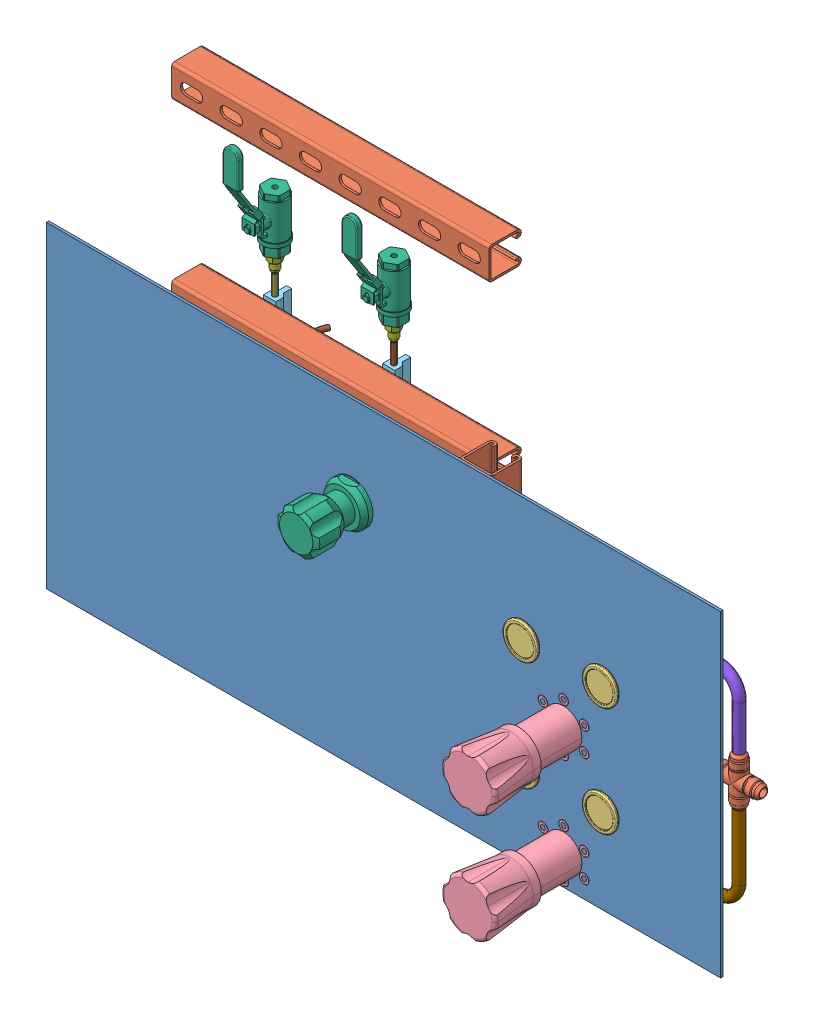
SolidWorks assembly N2_node, configuration Default. Lengths in mm.
Overall size (880 623.2 374.6).
79 component instances, 30 part files, 48 mates.
Components (placement in the parent):
- Pressure_panel-1: Pressure_panel [Default] at origin size (863.6 406.4 3.17)
- SS-2650-08-08-08-08-1: SS-2650-08-08-08-08 [5482K249] at (400.8501 -25.4 -51.435) size (81.9 81.9 19.05)
- 9780T219_VIBRATION-RESISTANT PRESSURE GAUGE-3: 9780T219_VIBRATION-RESISTANT PRESSURE GAUGE [9780T219] at (179.9381 -92.6228 8.636) x (-1 0 0) z (0 0 1) size (44.45 61.91 48.07)
- 9780T219_VIBRATION-RESISTANT PRESSURE GAUGE-4: 9780T219_VIBRATION-RESISTANT PRESSURE GAUGE [9780T219] at (281.5381 -92.6228 8.636) x (-1 0 0) z (0 0 1) size (44.45 61.91 48.07)
- PRV-1 & PRV-2 Assembly-1: PRV-1 & PRV-2 Assembly [Default] at (230.7381 -165.1 -104.521) size (144.32 78.02 230.14)
  - PRV-1&2_RSHN4-02-6-VVK-Swagelok-1: PRV-1&2_RSHN4-02-6-VVK-Swagelok [Default] at origin size (72 78.02 230.14)
  - 50715K802-1: 50715K802 [50715K802] at (39.556 0 53.086) x (1 0 0) z (0 0.0006 1) size (55.21 25.66 22.23)
  - 50715K802-2: 50715K802 [50715K802] at (-39.556 0 53.086) x (-1 0 0) z (0 -0.0006 -1) size (55.21 25.66 22.23)
- PRV-3 Assembly-1: PRV-3 Assembly [Default] at (-40.8559 88.9 -138.049) x (-1 0 0) z (0 0 1) size (139.78 55.88 212.09)
  - KCY1JPA412A20000_PRT_29-1: KCY1JPA412A20000_PRT_29 [Default] at origin size (56.39 55.88 212.09)
  - 51205K317_EXTREME-PRESSURE 316 SS THREADED PIPE FITTING-1: 51205K317_EXTREME-PRESSURE 316 SS THREADED PIPE FITTING [51205K317] at (-34.807 0 86.614) x (-1 0 0) z (0 0.601506 -0.798868) size (42.93 32.74 28.57)
  - 50715K802-1: 50715K802 [50715K802] at (-59.826 0 86.614) x (-1 0 0) z (0 -0.969103 0.246658) size (55.21 25.66 22.23)
  - 50715K163_TYPE 316 SS 37 DEGREE FLARED TUBE FITTING-1: 50715K163_TYPE 316 SS 37 DEGREE FLARED TUBE FITTING [50715K163] at (29.187 0 86.614) size (36.32 18.33 15.88)
- IPA_N2_manifold_1-1: IPA_N2_manifold_1 [Default] at (13.0485 -6.0223 -0.8427) x (1 0 0) z (0 0.258819 0.965926) size (242.25 185.67 41.98)
  - 50715K802-1: 50715K802 [50715K802] at (18.6216 -140.563 -90.0408) x (1 0 0) z (0 -0.539316 0.842104) size (55.21 25.66 22.23)
  - 5627K623_BRASS MANIFOLD WITH OUTLETS ON ONE SIDE-1: 5627K623_BRASS MANIFOLD WITH OUTLETS ON ONE SIDE [5627K623] at (-69.8974 -140.563 -90.0408) x (0 0 -1) z (1 0 0) size (38.1 38.1 158.75)
  - 4443K732_HIGH-PRESSURE 316 SS THREADED PIPE FITTING-1: 4443K732_HIGH-PRESSURE 316 SS THREADED PIPE FITTING [4443K732] at (-50.8474 -125.958 -90.0408) x (0 -1 0) z (0.415851 0 0.909433) size (19.05 20.24 17.88)
  - Pressure_sensor_standin-1: Pressure_sensor_standin [Default] at (-50.8474 -98.1907 -90.0408) x (0 -1 0) z (0.600596 0 -0.799553) size (123.69 32.03 28.45)
  - HPRV-500_PSV-1,2-1: HPRV-500_PSV-1,2 [Default] at (-12.7474 26.061 -90.0408) x (0.240643 0 0.970614) z (0 -1 0) size (31.75 35.92 128.52)
  - 5482K122_PRECISION AN 37 DEGREE FLARED TUBE FITTING-1: 5482K122_PRECISION AN 37 DEGREE FLARED TUBE FITTING [5482K122] at (-88.9474 -114.0708 -90.0408) x (0 1 0) z (0 0 1) size (45.71 22 19.05)
  - 5482K162_PRECISION AN 37 DEGREE FLARED TUBE FITTING-1: 5482K162_PRECISION AN 37 DEGREE FLARED TUBE FITTING [5482K162] at (-88.9474 -85.5844 -90.0408) x (0 1 0) z (-0.483856 0 -0.875148) size (34.61 12.75 12.75)
  - 48805K460_PRECISION EXTREME-PRESSURE 316SS PIPE FITTING-1: 48805K460_PRECISION EXTREME-PRESSURE 316SS PIPE FITTING [48805K46] at (-12.7474 -110.464 -90.0408) x (0 -1 0) z (-0.516882 0 0.856057) size (42.93 33 28.57)
  - 50715K802-2: 50715K802 [50715K802] at (-158.4164 -140.563 -90.0408) x (-1 0 0) z (0 -0.862244 -0.506493) size (55.21 25.66 22.23)
  - 5482K162_PRECISION AN 37 DEGREE FLARED TUBE FITTING-3: 5482K162_PRECISION AN 37 DEGREE FLARED TUBE FITTING [5482K162] at (-127.0474 -85.5844 -90.0408) x (0 1 0) z (-0.483856 0 -0.875148) size (34.61 12.75 12.75)
  - 5482K122_PRECISION AN 37 DEGREE FLARED TUBE FITTING-2: 5482K122_PRECISION AN 37 DEGREE FLARED TUBE FITTING [5482K122] at (-127.0474 -114.0708 -90.0408) x (0 1 0) z (0 0 1) size (45.71 22 19.05)
- 9780T219_VIBRATION-RESISTANT PRESSURE GAUGE-5: 9780T219_VIBRATION-RESISTANT PRESSURE GAUGE [9780T219] at (-152.4 21.6772 8.636) size (44.45 61.91 48.07) (suppressed, hidden)
- 9780T219_VIBRATION-RESISTANT PRESSURE GAUGE-6: 9780T219_VIBRATION-RESISTANT PRESSURE GAUGE [9780T219] at (-76.2 21.6772 8.636) size (44.45 61.91 48.07) (suppressed, hidden)
- PRV-1 & PRV-2 Assembly-2: PRV-1 & PRV-2 Assembly [Default] at (-127 -76.1799 -125.3) x (-1 0 0) z (0 0 1) size (144.32 78.02 230.14) (suppressed, hidden)
  - PRV-1&2_RSHN4-02-6-VVK-Swagelok-1: PRV-1&2_RSHN4-02-6-VVK-Swagelok [Default] at origin size (72 78.02 230.14)
  - 50715K802-1: 50715K802 [50715K802] at (39.556 0 53.086) x (1 0 0) z (0 0.0006 1) size (55.21 25.66 22.23)
  - 50715K802-2: 50715K802 [50715K802] at (-39.556 0 53.086) x (-1 0 0) z (0 -0.0006 -1) size (55.21 25.66 22.23)
- N2_pilot_manifold-1: N2_pilot_manifold [Default] at (22.6847 -98.425 -10.16) size (226.06 32.55 141.21)
  - 5784T133_ASME-CODE NCKL-PLTD BRASS POP-SAFETY VALVE-1: 5784T133_ASME-CODE NCKL-PLTD BRASS POP-SAFETY VALVE [5784T133] at (-394.716 187.325 -41.275) x (0 0.086231 0.996275) z (0 -0.996275 0.086231) size (19.05 66.64 20.16)
  - 4839K732_TYPE 303 STAINLESS STEEL MANIFOLD-1: 4839K732_TYPE 303 STAINLESS STEEL MANIFOLD [4839K732] at (-331.7875 187.325 -41.275) x (0 -1 0) z (1 0 0) size (31.75 32.09 149.63)
  - 50715K164_TYPE 316 SS 37 DEGREE FLARED TUBE FITTING-1: 50715K164_TYPE 316 SS 37 DEGREE FLARED TUBE FITTING [50715K164] at (-253.111 187.325 -41.275) size (36.97 22 19.05)
  - 5361K320_TYPE 304 STAINLESS STEEL BARBED HOSE FITTING-1: 5361K320_TYPE 304 STAINLESS STEEL BARBED HOSE FITTING [5361K32] at (-387.35 187.325 -63.5) x (-0.53642 -0.843951 0) z (0 0 -1) size (14.29 16.5 47.66)
  - Pressure_sensor_standin-1: Pressure_sensor_standin [Default] at (-276.225 187.325 -71.374) x (0 0 1) z (-0.999827 -0.018586 0) size (123.69 32.03 28.45)
  - 5361K320_TYPE 304 STAINLESS STEEL BARBED HOSE FITTING-2: 5361K320_TYPE 304 STAINLESS STEEL BARBED HOSE FITTING [5361K32] at (-365.125 187.325 -63.5) x (-0.53642 -0.843951 0) z (0 0 -1) size (14.29 16.5 47.66)
  - 5361K320_TYPE 304 STAINLESS STEEL BARBED HOSE FITTING-3: 5361K320_TYPE 304 STAINLESS STEEL BARBED HOSE FITTING [5361K32] at (-342.9 187.325 -63.5) x (-0.53642 -0.843951 0) z (0 0 -1) size (14.29 16.5 47.66)
  - 5361K320_TYPE 304 STAINLESS STEEL BARBED HOSE FITTING-4: 5361K320_TYPE 304 STAINLESS STEEL BARBED HOSE FITTING [5361K32] at (-320.675 187.325 -63.5) x (-0.53642 -0.843951 0) z (0 0 -1) size (14.29 16.5 47.66)
  - 5361K320_TYPE 304 STAINLESS STEEL BARBED HOSE FITTING-5: 5361K320_TYPE 304 STAINLESS STEEL BARBED HOSE FITTING [5361K32] at (-298.45 187.325 -63.5) x (-0.53642 -0.843951 0) z (0 0 -1) size (14.29 16.5 47.66)
- 3310T530_STRUT CHANNEL_16-1: 3310T530_STRUT CHANNEL_16 [3310T53] at (114.6011 203.2 0) x (0 0 1) z (0 1 0) size (41.27 41.27 406.4)
- 008T012-1: 008T012 [Default] at (114.6011 88.9 -51.435) x (0 1 0) z (-1 0 0) size (23.88 34.04 44.45)
- 008T012-2: 008T012 [Default] at (114.6011 -165.1 -51.435) x (0 1 0) z (-1 0 0) size (23.88 34.04 44.45)
- 9780T219_VIBRATION-RESISTANT PRESSURE GAUGE-9: 9780T219_VIBRATION-RESISTANT PRESSURE GAUGE [9780T219] at (281.5381 47.0772 8.636) x (-1 0 0) z (0 0 1) size (44.45 61.91 48.07)
- 9780T219_VIBRATION-RESISTANT PRESSURE GAUGE-10: 9780T219_VIBRATION-RESISTANT PRESSURE GAUGE [9780T219] at (179.9381 47.0772 8.636) x (-1 0 0) z (0 0 1) size (44.45 61.91 48.07)
- 008T012-4: 008T012 [Default] at (114.6011 -25.4 -51.435) x (0 1 0) z (-1 0 0) size (23.88 34.04 44.45)
- PRV-1 & PRV-2 Assembly-4: PRV-1 & PRV-2 Assembly [Default] at (230.7381 -25.4 -104.521) size (144.32 78.02 230.14)
  - PRV-1&2_RSHN4-02-6-VVK-Swagelok-1: PRV-1&2_RSHN4-02-6-VVK-Swagelok [Default] at origin size (72 78.02 230.14)
  - 50715K802-1: 50715K802 [50715K802] at (39.556 0 53.086) x (1 0 0) z (0 0.0006 1) size (55.21 25.66 22.23)
  - 50715K802-2: 50715K802 [50715K802] at (-39.556 0 53.086) x (-1 0 0) z (0 -0.0006 -1) size (55.21 25.66 22.23)
- 3310T530_STRUT CHANNEL_16-2: 3310T530_STRUT CHANNEL_16 [3310T53] at (93.9636 157.1625 -38.1) x (0 0 1) z (1 0 0) size (41.27 41.27 406.4)
- LOX_N2_manifold_1-1: LOX_N2_manifold_1 [Default] at (-139.3515 133.6777 -0.8427) x (1 0 0) z (0 0.258819 0.965926) size (242.25 185.67 41.98)
  - 50715K802-1: 50715K802 [50715K802] at (18.6216 -140.563 -90.0408) x (1 0 0) z (0 -0.539316 0.842104) size (55.21 25.66 22.23)
  - 5627K623_BRASS MANIFOLD WITH OUTLETS ON ONE SIDE-1: 5627K623_BRASS MANIFOLD WITH OUTLETS ON ONE SIDE [5627K623] at (-69.8974 -140.563 -90.0408) x (0 0 -1) z (1 0 0) size (38.1 38.1 158.75)
  - 4443K732_HIGH-PRESSURE 316 SS THREADED PIPE FITTING-1: 4443K732_HIGH-PRESSURE 316 SS THREADED PIPE FITTING [4443K732] at (-50.8474 -125.958 -90.0408) x (0 -1 0) z (0.415851 0 0.909433) size (19.05 20.24 17.88)
  - Pressure_sensor_standin-1: Pressure_sensor_standin [Default] at (-50.8474 -98.1907 -90.0408) x (0 -1 0) z (0.600596 0 -0.799553) size (123.69 32.03 28.45)
  - HPRV-500_PSV-1,2-1: HPRV-500_PSV-1,2 [Default] at (-12.7474 26.061 -90.0408) x (0.240643 0 0.970614) z (0 -1 0) size (31.75 35.92 128.52)
  - 5482K122_PRECISION AN 37 DEGREE FLARED TUBE FITTING-1: 5482K122_PRECISION AN 37 DEGREE FLARED TUBE FITTING [5482K122] at (-88.9474 -114.0708 -90.0408) x (0 1 0) z (0 0 1) size (45.71 22 19.05)
  - 5482K162_PRECISION AN 37 DEGREE FLARED TUBE FITTING-1: 5482K162_PRECISION AN 37 DEGREE FLARED TUBE FITTING [5482K162] at (-88.9474 -85.5844 -90.0408) x (0 1 0) z (-0.483856 0 -0.875148) size (34.61 12.75 12.75)
  - 48805K460_PRECISION EXTREME-PRESSURE 316SS PIPE FITTING-1: 48805K460_PRECISION EXTREME-PRESSURE 316SS PIPE FITTING [48805K46] at (-12.7474 -110.464 -90.0408) x (0 -1 0) z (-0.516882 0 0.856057) size (42.93 33 28.57)
  - 50715K802-2: 50715K802 [50715K802] at (-158.4164 -140.563 -90.0408) x (-1 0 0) z (0 -0.862244 -0.506493) size (55.21 25.66 22.23)
  - 4757T730_HIGH-PRESSURE BRASS THREADED PIPE FITTING-1: 4757T730_HIGH-PRESSURE BRASS THREADED PIPE FITTING [4757T73] at (-127.0474 -122.021 -90.0408) x (0 1 0) z (0.804983 0 0.593298) size (19.81 20.16 17.46)
- 004T008-1: 004T008 [Default] at (-228.2989 157.1625 -86.233) x (1 0 0) z (0 1 0) size (15.75 24.89 44.45)
- 004T008-2: 004T008 [Default] at (-75.8989 157.1625 -86.233) x (1 0 0) z (0 1 0) size (15.75 24.89 44.45)
- HV-1,2-3: HV-1,2 [Default] at (-147.2516 235.6926 -190.7689) x (-0.983779 0 -0.179384) z (0.179384 0 -0.983779) size (44.38 176.24 77.79)
  - 47275K410_ULTRA-HIGH-PRESSURE 316SS BALL VALVE-1: 47275K410_ULTRA-HIGH-PRESSURE 316SS BALL VALVE [47275K41] at (-88.9474 28.7849 -90.0408) x (-0.983779 0 0.179384) z (0 -1 0) size (31.75 73.28 141.48)
  - 5482K118_PRECISION AN 37 DEGREE FLARED TUBE FITTING-1: 5482K118_PRECISION AN 37 DEGREE FLARED TUBE FITTING [5482K118] at (-88.9474 -13.4426 -90.0408) x (0 -1 0) z (0.141466 0 0.989943) size (44.92 16.5 14.29)
- HV-1,2-4: HV-1,2 [Default] at (-299.6516 235.6926 -190.7689) x (-0.983779 0 -0.179384) z (0.179384 0 -0.983779) size (44.38 176.24 77.79)
  - 47275K410_ULTRA-HIGH-PRESSURE 316SS BALL VALVE-1: 47275K410_ULTRA-HIGH-PRESSURE 316SS BALL VALVE [47275K41] at (-88.9474 28.7849 -90.0408) x (-0.983779 0 0.179384) z (0 -1 0) size (31.75 73.28 141.48)
  - 5482K118_PRECISION AN 37 DEGREE FLARED TUBE FITTING-1: 5482K118_PRECISION AN 37 DEGREE FLARED TUBE FITTING [5482K118] at (-88.9474 -13.4426 -90.0408) x (0 -1 0) z (0.141466 0 0.989943) size (44.92 16.5 14.29)
- Tube_1-N2_node-001-1: Tube_1-N2_node-001 [Default] at origin size (507.95 266.7 374.6)
  - Tube-500X010^Tube_1-N2_node-001-1: Tube-500X010^Tube_1-N2_node-001 [Tube .500in OD X .010in Wall] at (400.8501 5.5499 -51.435) x (0.707107 0 0.707107) z (0 1 0) size (264.89 264.89 89.7) (virtual)
  - Tube-500X010_1^Tube_1-N2_node-001-1: Tube-500X010_1^Tube_1-N2_node-001 [Tube .500in OD X .010in Wall] at (400.8501 -56.3499 -51.435) x (0.707107 0 0.707107) z (0 -1 0) size (87.17 87.17 115.1) (virtual)
  - Tube-500X010_2^Tube_1-N2_node-001-1: Tube-500X010_2^Tube_1-N2_node-001 [Tube .500in OD X .010in Wall] at (168.5761 -25.4 -51.435) x (0 0.707107 0.707107) z (-1 0 0) size (12.7 12.7 266.7) (virtual)
- Tube_2-N2_node-001-1: Tube_2-N2_node-001 [Default] at origin size (201.04 307.99 146.21)
  - Tube-250X010^Tube_2-N2_node-001-1: Tube-250X010^Tube_2-N2_node-001 [Tube .250in OD X .010in Wall] at (-75.8989 -100.1078 -68.8496) x (0.694747 0.186157 0.694747) z (0 0.965926 -0.258819) size (50.98 49.46 299.83) (virtual)
  - Tube-250X010_1^Tube_2-N2_node-001-1: Tube-250X010_1^Tube_2-N2_node-001 [Tube .250in OD X .010in Wall] at (-228.2989 204.7875 -86.233) x (0.707107 0 0.707107) z (0 -1 0) size (18.59 18.59 166.02) (virtual)
- 3310T530_STRUT CHANNEL_16-3: 3310T530_STRUT CHANNEL_16 [3310T53] at (93.9636 398.4625 -38.1) x (0 0 1) z (1 0 0) size (41.27 41.27 406.4)
Mates (geometry in assembly coordinates):
- Coincident24: coincident anti-aligned: plane of Pressure_panel-1 through (0 0 3.175) normal (0 0 1); circle of 9780T219_VIBRATION-RESISTANT PRESSURE GAUGE-3
- Parallel12: parallel anti-aligned: plane of 9780T219_VIBRATION-RESISTANT PRESSURE GAUGE-4 through (273.0631 -61.6665 -18.7643) normal (-1 0 0)
- Parallel13: parallel aligned: plane of PRV-1 & PRV-2 Assembly-1/PRV-1&2_RSHN4-02-6-VVK-Swagelok-1 through (266.7381 -165.1 20.691) normal (1 0 0)
- Distance4: distance = 38.1 mm anti-aligned: plane of 9780T219_VIBRATION-RESISTANT PRESSURE GAUGE-3 through (183.0543 -98.0203 -29.718) normal (0 -1 0); plane of PRV-1 & PRV-2 Assembly-1/PRV-1&2_RSHN4-02-6-VVK-Swagelok-1 through (230.7381 -136.1203 -51.435) normal (0 1 0)
- Parallel18: parallel aligned: plane of SS-2650-08-08-08-08-1 through (400.8501 -25.4 -51.435) normal (0 0 1)
- Distance9: distance = 50.8 mm anti-aligned: plane of 9780T219_VIBRATION-RESISTANT PRESSURE GAUGE-3 through (179.9381 -92.6228 8.636) normal (-1 0 0); plane of PRV-1 & PRV-2 Assembly-1/PRV-1&2_RSHN4-02-6-VVK-Swagelok-1 through (230.7381 -165.1 -104.521) normal (1 0 0)
- Coincident69: coincident anti-aligned: plane of Pressure_panel-1 through (0 0 0) normal (0 0 -1); plane of 3310T530_STRUT CHANNEL_16-1 through (131.7779 -203.2 0) normal (0 0 1)
- Coincident74: coincident aligned: plane of Pressure_panel-1 through (-431.8 -203.2 3.175) normal (0 -1 0); plane of 3310T530_STRUT CHANNEL_16-1 through (130.1904 -203.2 -36.2268) normal (0 -1 0)
- Coincident72: coincident anti-aligned: plane of 3310T530_STRUT CHANNEL_16-1 through (99.0119 -203.2 -41.275) normal (0 0 -1); plane of 008T012-1 through (92.3761 100.838 -41.275) normal (0 0 1)
- Coincident75: coincident aligned: plane of 008T012-1 through (136.8261 88.9 -51.435) normal (1 0 0); plane of 008T012-2 through (136.8261 -165.1 -51.435) normal (1 0 0)
- Coincident76: coincident aligned: plane of 008T012-1 through (92.3761 85.725 -75.311) normal (0 0 -1); plane of 008T012-2 through (92.3761 -168.275 -75.311) normal (0 0 -1)
- Distance21: distance = 1.5875 mm aligned: plane of 008T012-1 through (136.8261 88.9 -51.435) normal (1 0 0); plane of 3310T530_STRUT CHANNEL_16-1 through (135.2386 -203.2 -36.2268) normal (1 0 0)
- Coincident84: coincident aligned: plane of Pressure_panel-1 through (431.8 203.2 3.175) normal (1 0 0); plane of SS-2650-08-08-08-08-1 through (431.8 -25.4 -51.435) normal (1 0 0)
- Concentric46: concentric anti-aligned: cone of PRV-1 & PRV-2 Assembly-1/PRV-1&2_RSHN4-02-6-VVK-Swagelok-1 through (259.2268 -165.1 -51.435) axis (-1 0 0); cylinder of 008T012-2 through (92.3761 -165.1 -51.435) axis (1 0 0) radius 6.35
- Distance23: distance = 107.95 mm aligned: plane of SS-2650-08-08-08-08-1 through (400.8501 -25.4 -51.435) normal (1 0 0); plane of PRV-1 & PRV-2 Assembly-1/50715K802-1 through (292.9001 -165.1 -51.435) normal (1 0 0)
- Concentric47: concentric aligned: cylinder of IPA_N2_manifold_1-1/5627K623_BRASS MANIFOLD WITH OUTLETS ON ONE SIDE-1 through (31.6542 -165.1 -51.435) axis (1 0 0) radius 9.1281; cylinder of 008T012-2 through (92.3761 -165.1 -51.435) axis (1 0 0) radius 6.35
- Distance24: distance = 31.75 mm anti-aligned: plane of 008T012-2 through (136.8261 -165.1 -51.435) normal (1 0 0); plane of PRV-1 & PRV-2 Assembly-1/50715K802-2 through (168.5761 -165.1 -51.435) normal (-1 0 0)
- Concentric48: concentric aligned: cylinder of PRV-3 Assembly-1/50715K802-1 through (41.5761 88.9 -51.435) axis (1 0 0) radius 4.953; cylinder of 008T012-1 through (92.3761 88.9 -51.435) axis (1 0 0) radius 6.35
- Parallel37: parallel aligned: plane of N2_pilot_manifold-1 through (22.6847 -98.425 -10.16) normal (0 1 0)
- Concentric49: concentric anti-aligned: cylinder of PRV-3 Assembly-1/50715K163_TYPE 316 SS 37 DEGREE FLARED TUBE FITTING-1 through (-51.8819 88.9 -51.435) axis (1 0 0) radius 7.1437; cylinder of N2_pilot_manifold-1/50715K164_TYPE 316 SS 37 DEGREE FLARED TUBE FITTING-1 through (-248.7143 88.9 -51.435) axis (-1 0 0) radius 7.1437
- Distance27: distance = 38.1 mm anti-aligned: plane of Pressure_panel-1 through (0 0 0) normal (0 0 -1); plane of 3310T530_STRUT CHANNEL_16-2 through (-312.4364 139.9857 -38.1) normal (0 0 1)
- Distance35: distance = 25.4 mm aligned: plane of Pressure_panel-1 through (-431.8 203.2 3.175) normal (0 1 0); plane of 3310T530_STRUT CHANNEL_16-2 through (-312.4364 177.8 -74.3268) normal (0 1 0)
- Coincident93: coincident anti-aligned: plane of 3310T530_STRUT CHANNEL_16-1 through (93.9636 -203.2 -36.2268) normal (-1 0 0); plane of 3310T530_STRUT CHANNEL_16-2 through (93.9636 141.5733 -74.3268) normal (1 0 0)
- Parallel38: parallel anti-aligned: plane of PRV-3 Assembly-1 through (-40.8559 88.9 -138.049) normal (0 -1 0)
- Concentric50: concentric anti-aligned: cylinder of PRV-1 & PRV-2 Assembly-4/50715K802-2 through (213.7881 -25.4 -51.435) axis (1 0 0) radius 9.525; cylinder of LOX_N2_manifold_1-1/50715K802-1 through (-143.3359 -25.4 -51.435) axis (-1 0 0) radius 9.525
- Parallel39: parallel aligned: plane of IPA_N2_manifold_1-1/5627K623_BRASS MANIFOLD WITH OUTLETS ON ONE SIDE-1 through (22.5261 -188.4314 -64.9054) normal (0 -0.258819 -0.965926); plane of LOX_N2_manifold_1-1/5627K623_BRASS MANIFOLD WITH OUTLETS ON ONE SIDE-1 through (-129.8739 -48.7314 -64.9054) normal (0 -0.258819 -0.965926)
- Distance28: distance = 38.1 mm: plane of PRV-1 & PRV-2 Assembly-1 through (230.7381 -165.1 -104.521) normal (0 1 0); line of Pressure_panel-1 through (-431.8 -203.2 3.175) axis (1 0 0)
- Angle1: planar angle = 0.261799 rad aligned: plane of IPA_N2_manifold_1-1/5627K623_BRASS MANIFOLD WITH OUTLETS ON ONE SIDE-1 through (22.5261 -188.4314 -64.9054) normal (0 -0.258819 -0.965926); plane of Pressure_panel-1 through (0 0 0) normal (0 0 -1)
- Coincident96: coincident anti-aligned: plane of 3310T530_STRUT CHANNEL_16-2 through (-312.4364 172.7518 -79.375) normal (0 0 -1); plane of 004T008-1 through (-220.4249 179.3875 -79.375) normal (0 0 1)
- Distance29: distance = 1.5875 mm aligned: plane of 3310T530_STRUT CHANNEL_16-2 through (-312.4364 177.8 -74.3268) normal (0 1 0); plane of 004T008-1 through (-228.2989 179.3875 -86.233) normal (0 1 0)
- Coincident98: coincident anti-aligned: plane of LOX_N2_manifold_1-1/5482K122_PRECISION AN 37 DEGREE FLARED TUBE FITTING-1 through (-228.2989 0.1895 -58.2917) normal (-1 0 0); plane of 004T008-1 through (-228.2989 157.1625 -86.233) normal (1 0 0)
- Distance30: distance = 38.1 mm anti-aligned: plane of IPA_N2_manifold_1-1/50715K802-1 through (54.2761 -165.1 -51.435) normal (1 0 0); plane of 008T012-2 through (92.3761 -165.1 -51.435) normal (-1 0 0)
- Coincident101: coincident aligned: plane of 004T008-1 through (-231.4739 179.3875 -104.267) normal (0 0 -1); plane of 004T008-2 through (-79.0739 179.3875 -104.267) normal (0 0 -1)
- Coincident102: coincident aligned: plane of 004T008-1 through (-228.2989 179.3875 -86.233) normal (0 1 0); plane of 004T008-2 through (-75.8989 179.3875 -86.233) normal (0 1 0)
- Coincident103: coincident anti-aligned: plane of IPA_N2_manifold_1-1/5482K122_PRECISION AN 37 DEGREE FLARED TUBE FITTING-1 through (-75.8989 -139.5105 -58.2917) normal (-1 0 0); plane of 004T008-2 through (-75.8989 157.1625 -86.233) normal (1 0 0)
- Concentric51: concentric anti-aligned: cylinder of 004T008-2 through (-75.8989 179.3875 -86.233) axis (0 -1 0) radius 3.175; cylinder of HV-1,2-3/5482K118_PRECISION AN 37 DEGREE FLARED TUBE FITTING-1 through (-75.8989 239.7125 -86.233) axis (0 1 0) radius 5.5563
- Concentric52: concentric anti-aligned: cylinder of 004T008-1 through (-228.2989 179.3875 -86.233) axis (0 -1 0) radius 3.175; cylinder of HV-1,2-4/5482K118_PRECISION AN 37 DEGREE FLARED TUBE FITTING-1 through (-228.2989 239.7125 -86.233) axis (0 1 0) radius 5.5563
- Coincident106: coincident aligned: plane of HV-1,2-3/47275K410_ULTRA-HIGH-PRESSURE 316SS BALL VALVE-1 through (-75.8989 299.4025 -86.233) normal (0 1 0); plane of HV-1,2-4/47275K410_ULTRA-HIGH-PRESSURE 316SS BALL VALVE-1 through (-228.2989 299.4025 -86.233) normal (0 1 0)
- Distance31: distance = 152.4 mm aligned: plane of 004T008-1 through (-236.1729 179.3875 -79.375) normal (-1 0 0); plane of 004T008-2 through (-83.7729 179.3875 -79.375) normal (-1 0 0)
- Distance32: distance = 254 mm aligned: plane of 008T012-1 through (92.3761 100.838 -51.435) normal (0 1 0); plane of 008T012-2 through (92.3761 -153.162 -51.435) normal (0 1 0)
- Distance34: distance = 12.7 mm aligned: plane of PRV-3 Assembly-1/50715K802-1 through (41.5761 88.9 -51.435) normal (1 0 0); plane of IPA_N2_manifold_1-1/50715K802-1 through (54.2761 -165.1 -51.435) normal (1 0 0)
- Distance33: distance = 25.4 mm anti-aligned: plane of 004T008-1 through (-228.2989 179.3875 -86.233) normal (0 1 0); plane of HV-1,2-4/5482K118_PRECISION AN 37 DEGREE FLARED TUBE FITTING-1 through (-228.2989 204.7875 -86.233) normal (0 -1 0)
- Parallel43: parallel aligned: plane of HV-1,2-3/47275K410_ULTRA-HIGH-PRESSURE 316SS BALL VALVE-1 through (-75.8989 264.4775 -86.233) normal (0 0 1)
- Parallel44: parallel aligned: plane of HV-1,2-4/47275K410_ULTRA-HIGH-PRESSURE 316SS BALL VALVE-1 through (-228.2989 264.4775 -86.233) normal (0 0 1)
- Concentric53: concentric aligned: cylinder of SS-2650-08-08-08-08-1 through (400.8501 -25.4 -51.435) axis (-1 0 0) radius 9.525; cylinder of PRV-1 & PRV-2 Assembly-4/50715K802-1 through (247.6881 -25.4 -51.435) axis (-1 0 0) radius 9.525
- Coincident112: coincident aligned: plane of 3310T530_STRUT CHANNEL_16-2 through (93.9636 141.5733 -74.3268) normal (1 0 0); plane of 3310T530_STRUT CHANNEL_16-3 through (93.9636 382.8732 -74.3268) normal (1 0 0)
- Coincident113: coincident aligned: plane of 3310T530_STRUT CHANNEL_16-2 through (-312.4364 139.9857 -38.1) normal (0 0 1); plane of 3310T530_STRUT CHANNEL_16-3 through (-312.4364 381.2858 -38.1) normal (0 0 1)
- Distance36: distance = 241.3 mm aligned: plane of 3310T530_STRUT CHANNEL_16-2 through (-312.4364 177.8 -74.3268) normal (0 1 0); plane of 3310T530_STRUT CHANNEL_16-3 through (-312.4364 419.1 -74.3268) normal (0 1 0)
